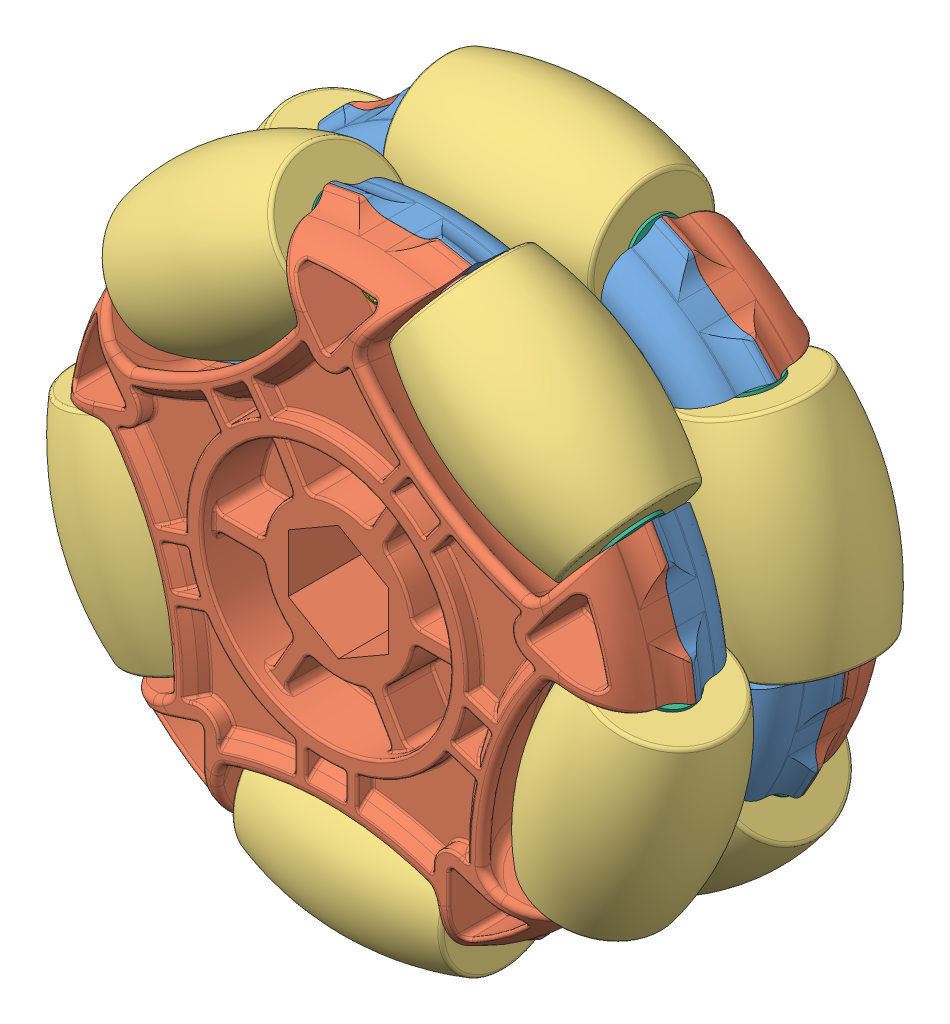
SolidWorks assembly 3_25_Omni-Directional_Wheel_217-4775, configuration Default. Lengths in mm.
Overall size (94.7 90.19 43.57).
63 component instances, 7 part files, 0 mates.
Components (placement in the parent):
- 217-4775-001 Rev5-1: 217-4775-001 Rev5 [Default] at origin size (75.36 74.93 19.12)
- 217-4775-003 Rev5-1: 217-4775-003 Rev5 [Default] at (0 0 -9.525) x (1 0 0) z (0 0 -1) size (75.36 72.49 19.19)
- 217-4775-004 Rev1_Smooth-1: 217-4775-004 Rev1_Smooth [Default] at (-13.5413 31.12 -9.525) x (1 0 0) z (0 0.745117 -0.666934) size (26.67 20.3 20.3)
- 217-4775-004 Rev1_Smooth-2: 217-4775-004 Rev1_Smooth [Default] at (-13.5413 -31.12 9.525) x (1 0 0) z (0 1 0) size (26.67 20.3 20.3)
- 217-4775-005 Rev1-1: 217-4775-005 Rev1 [Default] at (-0.1613 31.12 -9.525) x (0 -0.052651 -0.998613) z (1 0 0) size (3 3 31.95)
- 217-4775-005 Rev1-2: 217-4775-005 Rev1 [Default] at (-0.1613 -31.12 9.525) x (0 0.477136 -0.878829) z (1 0 0) size (3 3 31.95)
- 217-4775-005 Rev1-3: 217-4775-005 Rev1 [Default] at (-29.6467 9.4632 -9.525) x (0.050074 -0.01627 -0.998613) z (0.309017 0.951057 0) size (3 3 31.95)
- 217-4775-005 Rev1-4: 217-4775-005 Rev1 [Default] at (-18.1614 -25.2714 -9.525) x (0.030947 0.042595 -0.998613) z (-0.809017 0.587785 0) size (3 3 31.95)
- 217-4775-005 Rev1-5: 217-4775-005 Rev1 [Default] at (18.4223 -25.0818 -9.525) x (-0.030947 0.042595 -0.998613) z (-0.809017 -0.587785 0) size (3 3 31.95)
- 217-4775-005 Rev1-6: 217-4775-005 Rev1 [Default] at (29.547 9.77 -9.525) x (-0.050074 -0.01627 -0.998613) z (0.309017 -0.951057 0) size (3 3 31.95)
- 217-4775-004 Rev1_Smooth-3: 217-4775-004 Rev1_Smooth [Default] at (-33.7814 -3.2619 -9.525) x (0.309017 0.951057 0) z (-0.708648 0.230254 -0.666934) size (26.67 20.3 20.3)
- 217-4775-004 Rev1_Smooth-4: 217-4775-004 Rev1_Smooth [Default] at (-7.3368 -33.136 -9.525) x (-0.809017 0.587785 0) z (-0.437969 -0.602812 -0.666934) size (26.67 20.3 20.3)
- 217-4775-004 Rev1_Smooth-5: 217-4775-004 Rev1_Smooth [Default] at (29.247 -17.2173 -9.525) x (-0.809017 -0.587785 0) z (0.437969 -0.602812 -0.666934) size (26.67 20.3 20.3)
- 217-4775-004 Rev1_Smooth-6: 217-4775-004 Rev1_Smooth [Default] at (25.4124 22.4951 -9.525) x (0.309017 -0.951057 0) z (0.708648 0.230254 -0.666934) size (26.67 20.3 20.3)
- 217-4775-005 Rev1-7: 217-4775-005 Rev1 [Default] at (29.547 -9.77 9.525) x (-0.453783 0.147443 -0.878829) z (0.309017 0.951057 0) size (3 3 31.95)
- 217-4775-005 Rev1-8: 217-4775-005 Rev1 [Default] at (18.4223 25.0818 9.525) x (-0.280454 -0.386011 -0.878829) z (-0.809017 0.587785 0) size (3 3 31.95)
- 217-4775-005 Rev1-9: 217-4775-005 Rev1 [Default] at (-18.1614 25.2714 9.525) x (0.280454 -0.386011 -0.878829) z (-0.809017 -0.587785 0) size (3 3 31.95)
- 217-4775-005 Rev1-10: 217-4775-005 Rev1 [Default] at (-29.6467 -9.4632 9.525) x (0.453783 0.147443 -0.878829) z (0.309017 -0.951057 0) size (3 3 31.95)
- 217-4775-004 Rev1_Smooth-7: 217-4775-004 Rev1_Smooth [Default] at (25.4124 -22.4951 9.525) x (0.309017 0.951057 0) z (-0.951057 0.309017 0) size (26.67 20.3 20.3)
- 217-4775-004 Rev1_Smooth-8: 217-4775-004 Rev1_Smooth [Default] at (29.247 17.2173 9.525) x (-0.809017 0.587785 0) z (-0.587785 -0.809017 0) size (26.67 20.3 20.3)
- 217-4775-004 Rev1_Smooth-9: 217-4775-004 Rev1_Smooth [Default] at (-7.3368 33.136 9.525) x (-0.809017 -0.587785 0) z (0.587785 -0.809017 0) size (26.67 20.3 20.3)
- 217-4775-004 Rev1_Smooth-10: 217-4775-004 Rev1_Smooth [Default] at (-33.7814 3.2619 9.525) x (0.309017 -0.951057 0) z (0.951057 0.309017 0) size (26.67 20.3 20.3)
- 217-4775-007 Rev1-1: 217-4775-007 Rev1 [Default] at (-0.1913 31.12 -9.525) x (0 -0.721482 0.692433) z (-1 0 0) size (4.05 4.05 26.7)
- 217-4775-007 Rev1-2: 217-4775-007 Rev1 [Default] at (-29.656 9.4347 -9.525) x (0.68617 -0.22295 0.692433) z (-0.309017 -0.951057 0) size (4.05 4.05 26.7)
- 217-4775-007 Rev1-3: 217-4775-007 Rev1 [Default] at (-18.1371 -25.289 -9.525) x (0.424076 0.583691 0.692433) z (0.809017 -0.587785 0) size (4.05 4.05 26.7)
- 217-4775-007 Rev1-4: 217-4775-007 Rev1 [Default] at (18.4466 -25.0642 -9.525) x (-0.424076 0.583691 0.692433) z (0.809017 0.587785 0) size (4.05 4.05 26.7)
- 217-4775-007 Rev1-5: 217-4775-007 Rev1 [Default] at (29.5378 9.7985 -9.525) x (-0.68617 -0.22295 0.692433) z (-0.309017 0.951057 0) size (4.05 4.05 26.7)
- 217-4775-007 Rev1-6: 217-4775-007 Rev1 [Default] at (-18.1129 25.3067 9.525) x (-0.576222 0.793101 -0.197382) z (0.809017 0.587785 0) size (4.05 4.05 26.7)
- 217-4775-007 Rev1-7: 217-4775-007 Rev1 [Default] at (-29.6653 -9.4062 9.525) x (-0.932346 -0.302938 -0.197382) z (-0.309017 0.951057 0) size (4.05 4.05 26.7)
- 217-4775-007 Rev1-8: 217-4775-007 Rev1 [Default] at (-0.2213 -31.12 9.525) x (0 -0.980327 -0.197382) z (-1 0 0) size (4.05 4.05 26.7)
- 217-4775-007 Rev1-9: 217-4775-007 Rev1 [Default] at (29.5285 -9.827 9.525) x (0.932346 -0.302938 -0.197382) z (-0.309017 -0.951057 0) size (4.05 4.05 26.7)
- 217-4775-007 Rev1-10: 217-4775-007 Rev1 [Default] at (18.4709 25.0466 9.525) x (0.576222 0.793101 -0.197382) z (0.809017 -0.587785 0) size (4.05 4.05 26.7)
- 217-4775-003 Rev5-2: 217-4775-003 Rev5 [Default] at (0 0 9.525) size (75.36 72.49 19.19)
- 217-2584-009 Rev1-1: 217-2584-009 Rev1 [Default] at (29.247 -17.2173 -9.525) x (0.586309 -0.806985 0.070826) z (-0.041631 0.0573 0.997489) size (7 0.38 7)
- 217-2584-009 Rev1-2: 217-2584-009 Rev1 [Default] at (7.6705 32.8935 9.525) x (0.587762 0.808985 -0.008932) z (0.00525 0.007226 0.99996) size (7 0.38 7)
- 217-2584-009 Rev1-3: 217-2584-009 Rev1 [Default] at (33.7713 -3.231 -9.525) x (0.907415 0.294837 0.299448) z (-0.284792 -0.092534 0.954113) size (7 0.38 7)
- 217-2584-009 Rev1-4: 217-2584-009 Rev1 [Default] at (29.5544 16.9939 9.525) x (0.151982 0.209185 -0.965993) z (0.567797 0.781505 0.258567) size (7 0.38 7)
- 217-2584-009 Rev1-5: 217-2584-009 Rev1 [Default] at (-7.0293 33.3593 9.525) x (-0.151982 0.209185 -0.965993) z (-0.567797 0.781505 0.258567) size (7 0.38 7)
- 217-2584-009 Rev1-6: 217-2584-009 Rev1 [Default] at (-33.8988 3.6233 9.525) x (-0.245912 -0.079902 -0.965993) z (-0.918714 -0.298508 0.258567) size (7 0.38 7)
- 217-2584-009 Rev1-7: 217-2584-009 Rev1 [Default] at (-13.9213 -31.12 9.525) x (0 -0.258567 -0.965993) z (0 -0.965993 0.258567) size (7 0.38 7)
- 217-2584-009 Rev1-8: 217-2584-009 Rev1 [Default] at (25.295 -22.8565 9.525) x (0.245912 -0.079902 -0.965993) z (0.918714 -0.298508 0.258567) size (7 0.38 7)
- 217-2584-009 Rev1-9: 217-2584-009 Rev1 [Default] at (13.5087 31.12 -9.525) x (0 0.954113 0.299448) z (0 -0.299448 0.954113) size (7 0.38 7)
- 217-2584-009 Rev1-10: 217-2584-009 Rev1 [Default] at (-25.4224 22.4642 -9.525) x (-0.907415 0.294837 0.299448) z (0.284792 -0.092534 0.954113) size (7 0.38 7)
- 217-2584-009 Rev1-11: 217-2584-009 Rev1 [Default] at (-29.2207 -17.2364 -9.525) x (-0.560813 -0.771893 0.299448) z (0.176011 0.242258 0.954113) size (7 0.38 7)
- 217-2584-009 Rev1-12: 217-2584-009 Rev1 [Default] at (7.3631 -33.1168 -9.525) x (0.560813 -0.771893 0.299448) z (-0.176011 0.242258 0.954113) size (7 0.38 7)
- 217-2584-009 Rev1-13: 217-2584-009 Rev1 [Default] at (-28.9133 17.4597 9.525) x (-0.587762 0.808985 -0.008932) z (-0.00525 0.007226 0.99996) size (7 0.38 7)
- 217-2584-009 Rev1-14: 217-2584-009 Rev1 [Default] at (-25.5399 -22.1028 9.525) x (-0.951019 -0.309005 -0.008932) z (-0.008495 -0.00276 0.99996) size (7 0.38 7)
- 217-2584-009 Rev1-15: 217-2584-009 Rev1 [Default] at (13.1287 -31.12 9.525) x (0 -0.99996 -0.008932) z (0 -0.008932 0.99996) size (7 0.38 7)
- 217-2584-009 Rev1-16: 217-2584-009 Rev1 [Default] at (33.6539 2.8696 9.525) x (0.951019 -0.309005 -0.008932) z (0.008495 -0.00276 0.99996) size (7 0.38 7)
- 217-2584-009 Rev1-17: 217-2584-009 Rev1 [Default] at (25.4124 22.4951 -9.525) x (0.948668 0.308241 0.070826) z (-0.06736 -0.021887 0.997489) size (7 0.38 7)
- 217-2584-009 Rev1-18: 217-2584-009 Rev1 [Default] at (-13.5413 31.12 -9.525) x (0 0.997489 0.070826) z (0 -0.070826 0.997489) size (7 0.38 7)
- 217-2584-009 Rev1-19: 217-2584-009 Rev1 [Default] at (-33.7814 -3.2619 -9.525) x (-0.948668 0.308241 0.070826) z (0.06736 -0.021887 0.997489) size (7 0.38 7)
- 217-2584-009 Rev1-20: 217-2584-009 Rev1 [Default] at (-7.3368 -33.136 -9.525) x (-0.586309 -0.806985 0.070826) z (0.041631 0.0573 0.997489) size (7 0.38 7)
- 217-2584-007 Rev1_90116A020-1: 217-2584-007 Rev1_90116A020 [Default] at (-18.5152 25.484 -2.025) x (-0.859476 -0.511176 0) z (0 0 -1) size (4 4 11.7)
- 217-2584-007 Rev1_90116A020-2: 217-2584-007 Rev1_90116A020 [Default] at (-29.9583 9.734 2.025) x (0.995 0.099877 0) z (0 0 1) size (4 4 11.7)
- 217-2584-007 Rev1_90116A020-3: 217-2584-007 Rev1_90116A020 [Default] at (-18.5152 -25.484 2.025) x (0.212483 0.977165 0) z (0 0 1) size (4 4 11.7)
- 217-2584-007 Rev1_90116A020-4: 217-2584-007 Rev1_90116A020 [Default] at (18.5152 -25.484 2.025) x (-0.863678 0.504044 0) z (0 0 1) size (4 4 11.7)
- 217-2584-007 Rev1_90116A020-5: 217-2584-007 Rev1_90116A020 [Default] at (29.9583 9.734 2.025) x (-0.746266 -0.665648 0) z (0 0 1) size (4 4 11.7)
- 217-2584-007 Rev1_90116A020-6: 217-2584-007 Rev1_90116A020 [Default] at (0 31.5 2.025) x (0.40246 -0.915437 0) z (0 0 1) size (4 4 11.7)
- 217-2584-007 Rev1_90116A020-7: 217-2584-007 Rev1_90116A020 [Default] at (-29.9583 -9.734 -2.025) x (0.220564 -0.975372 0) z (0 0 -1) size (4 4 11.7)
- 217-2584-007 Rev1_90116A020-8: 217-2584-007 Rev1_90116A020 [Default] at (0 -31.5 -2.025) x (0.995792 -0.091637 0) z (0 0 -1) size (4 4 11.7)
- 217-2584-007 Rev1_90116A020-9: 217-2584-007 Rev1_90116A020 [Default] at (29.9583 -9.734 -2.025) x (0.394869 0.918737 0) z (0 0 -1) size (4 4 11.7)
- 217-2584-007 Rev1_90116A020-10: 217-2584-007 Rev1_90116A020 [Default] at (18.5152 25.484 -2.025) x (-0.75175 0.659448 0) z (0 0 -1) size (4 4 11.7)
